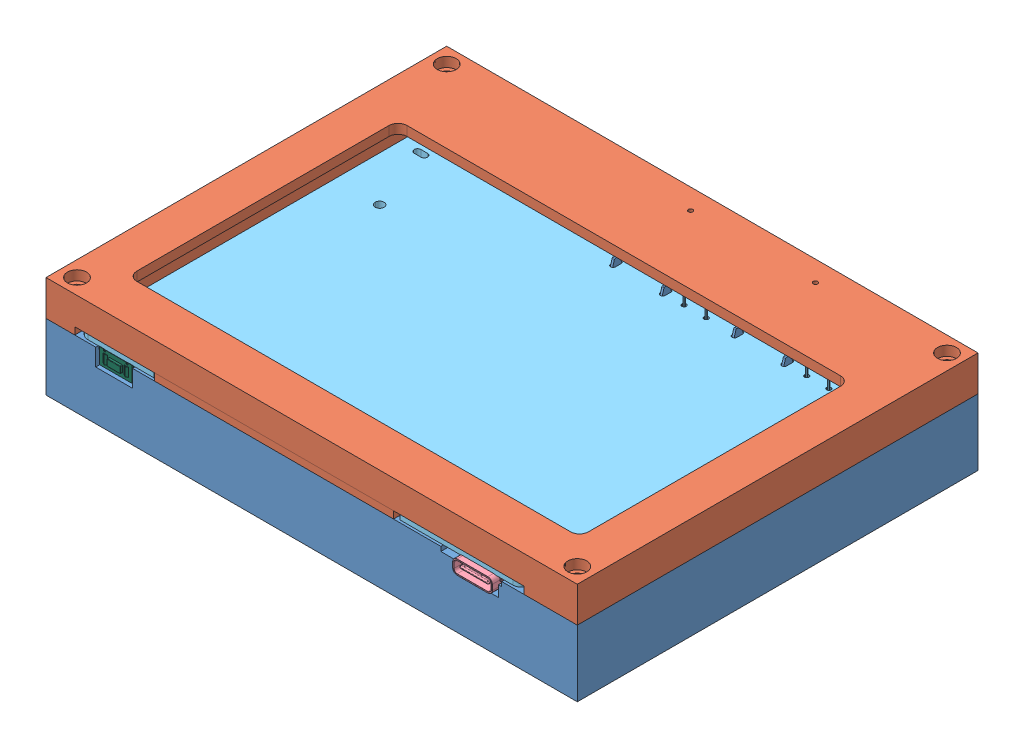
SolidWorks assembly 装配体2, configuration 默认. Lengths in mm. (continued)
Components (placement in the parent): (continued)
- 3D_board_2024-11-06-1: 3D_board_2024-11-06 [默认] at (-63.7814 -6.4105 44.7375) x (1 0 0) z (0 -1 0) size (99.97 100.01 16.2) (continued)
  - 3D_board_2024-11-06.step-1: 3D_board_2024-11-06.step [默认] at origin size (99.97 100.01 16.2) (continued)
    - iqks-C150.step-1: iqks-C150.step [默认] at (51.6811 -62.7701 1.5862) size (1.6 0.8 0.8)
      - C0603.step-1: C0603.step [默认] at origin size (1.6 0.8 0.8)
        - SOLID-10.step-1: SOLID-10.step [默认] at origin size (1.6 0.8 0.8)
    - iqks-C153.step-1: iqks-C153.step [默认] at (80.0102 -41.0211 1.5862) x (0 -1 0) z (0 0 1) size (1.6 0.8 0.8)
      - C0603.step-1: C0603.step [默认] at origin size (1.6 0.8 0.8)
        - SOLID-10.step-1: SOLID-10.step [默认] at origin size (1.6 0.8 0.8)
    - iqks-C15.step-1: iqks-C15.step [默认] at (71.7551 -65.8101 1.5862) x (0 1 0) z (0 0 1) size (1.6 0.8 0.8)
      - C0603.step-1: C0603.step [默认] at origin size (1.6 0.8 0.8)
        - SOLID-10.step-1: SOLID-10.step [默认] at origin size (1.6 0.8 0.8)
    - iqks-C16.step-1: iqks-C16.step [默认] at (83.1852 -65.8101 1.5862) x (0 1 0) z (0 0 1) size (1.6 0.8 0.8)
      - C0603.step-1: C0603.step [默认] at origin size (1.6 0.8 0.8)
        - SOLID-10.step-1: SOLID-10.step [默认] at origin size (1.6 0.8 0.8)
    - iqks-C38.step-1: iqks-C38.step [默认] at (85.7252 -65.8101 1.5862) x (0 1 0) z (0 0 1) size (1.6 0.8 0.8)
      - C0603.step-1: C0603.step [默认] at origin size (1.6 0.8 0.8)
        - SOLID-10.step-1: SOLID-10.step [默认] at origin size (1.6 0.8 0.8)
    - iqks-C39.step-1: iqks-C39.step [默认] at (97.1552 -65.8101 1.5862) x (0 1 0) z (0 0 1) size (1.6 0.8 0.8)
      - C0603.step-1: C0603.step [默认] at origin size (1.6 0.8 0.8)
        - SOLID-10.step-1: SOLID-10.step [默认] at origin size (1.6 0.8 0.8)
    - iqks-C17.step-1: iqks-C17.step [默认] at (26.6701 -67.3101 1.5862) x (0 -1 0) z (0 0 1) size (1.6 0.8 0.8)
      - C0603.step-1: C0603.step [默认] at origin size (1.6 0.8 0.8)
        - SOLID-10.step-1: SOLID-10.step [默认] at origin size (1.6 0.8 0.8)
    - iqks-C18.step-1: iqks-C18.step [默认] at (35.5601 -67.3101 1.5862) x (0 -1 0) z (0 0 1) size (1.6 0.8 0.8)
      - C0603.step-1: C0603.step [默认] at origin size (1.6 0.8 0.8)
        - SOLID-10.step-1: SOLID-10.step [默认] at origin size (1.6 0.8 0.8)
    - iqks-C50.step-1: iqks-C50.step [默认] at (12.065 -67.3101 1.5862) x (0 -1 0) z (0 0 1) size (1.6 0.8 0.8)
      - C0603.step-1: C0603.step [默认] at origin size (1.6 0.8 0.8)
        - SOLID-10.step-1: SOLID-10.step [默认] at origin size (1.6 0.8 0.8)
    - iqks-C51.step-1: iqks-C51.step [默认] at (20.955 -67.3101 1.5862) x (0 -1 0) z (0 0 1) size (1.6 0.8 0.8)
      - C0603.step-1: C0603.step [默认] at origin size (1.6 0.8 0.8)
        - SOLID-10.step-1: SOLID-10.step [默认] at origin size (1.6 0.8 0.8)
    - iqks-C22.step-1: iqks-C22.step [默认] at (17.78 -74.9301 1.5862) x (0 1 0) z (0 0 1) size (1.6 0.8 0.8)
      - C0603.step-1: C0603.step [默认] at origin size (1.6 0.8 0.8)
        - SOLID-10.step-1: SOLID-10.step [默认] at origin size (1.6 0.8 0.8)
    - iqks-C28.step-1: iqks-C28.step [默认] at (17.78 -71.1201 1.5862) x (0 -1 0) z (0 0 1) size (1.6 0.8 0.8)
      - C0603.step-1: C0603.step [默认] at origin size (1.6 0.8 0.8)
        - SOLID-10.step-1: SOLID-10.step [默认] at origin size (1.6 0.8 0.8)
    - iqks-C31.step-1: iqks-C31.step [默认] at (32.3851 -74.9301 1.5862) x (0 1 0) z (0 0 1) size (1.6 0.8 0.8)
      - C0603.step-1: C0603.step [默认] at origin size (1.6 0.8 0.8)
        - SOLID-10.step-1: SOLID-10.step [默认] at origin size (1.6 0.8 0.8)
    - iqks-C32.step-1: iqks-C32.step [默认] at (32.3851 -71.1201 1.5862) x (0 -1 0) z (0 0 1) size (1.6 0.8 0.8)
      - C0603.step-1: C0603.step [默认] at origin size (1.6 0.8 0.8)
        - SOLID-10.step-1: SOLID-10.step [默认] at origin size (1.6 0.8 0.8)
    - iqks-C113.step-1: iqks-C113.step [默认] at (53.8401 -57.5551 1.5862) x (0 1 0) z (0 0 1) size (1.6 0.8 0.8)
      - C0603.step-1: C0603.step [默认] at origin size (1.6 0.8 0.8)
        - SOLID-10.step-1: SOLID-10.step [默认] at origin size (1.6 0.8 0.8)
    - iqks-C116.step-1: iqks-C116.step [默认] at (38.1001 -59.0551 1.5862) x (0 1 0) z (0 0 1) size (1.6 0.8 0.8)
      - C0603.step-1: C0603.step [默认] at origin size (1.6 0.8 0.8)
        - SOLID-10.step-1: SOLID-10.step [默认] at origin size (1.6 0.8 0.8)
    - iqks-C25.step-1: iqks-C25.step [默认] at (63.1191 -60.9601 1.5862) x (-1 0 0) z (0 0 1) size (1.6 0.8 0.8)
      - C0603.step-1: C0603.step [默认] at origin size (1.6 0.8 0.8)
        - SOLID-10.step-1: SOLID-10.step [默认] at origin size (1.6 0.8 0.8)
    - iqks-C27.step-1: iqks-C27.step [默认] at (66.2941 -60.9601 1.5862) x (-1 0 0) z (0 0 1) size (1.6 0.8 0.8)
      - C0603.step-1: C0603.step [默认] at origin size (1.6 0.8 0.8)
        - SOLID-10.step-1: SOLID-10.step [默认] at origin size (1.6 0.8 0.8)
    - iqks-C129.step-1: iqks-C129.step [默认] at (58.0391 -59.6901 1.5862) x (0 1 0) z (0 0 1) size (1.6 0.8 0.8)
      - C0603.step-1: C0603.step [默认] at origin size (1.6 0.8 0.8)
        - SOLID-10.step-1: SOLID-10.step [默认] at origin size (1.6 0.8 0.8)
    - iqks-C154.step-1: iqks-C154.step [默认] at (60.3251 -50.8001 1.5862) x (0 -1 0) z (0 0 1) size (1.6 0.8 0.8)
      - C0603.step-1: C0603.step [默认] at origin size (1.6 0.8 0.8)
        - SOLID-10.step-1: SOLID-10.step [默认] at origin size (1.6 0.8 0.8)
    - iqks-C138.step-1: iqks-C138.step [默认] at (85.0902 -48.6411 1.5862) size (1.6 0.8 0.8)
      - C0603.step-1: C0603.step [默认] at origin size (1.6 0.8 0.8)
        - SOLID-10.step-1: SOLID-10.step [默认] at origin size (1.6 0.8 0.8)
    - iqks-C139.step-1: iqks-C139.step [默认] at (84.7092 -51.8161 1.5862) x (0 1 0) z (0 0 1) size (1.6 0.8 0.8)
      - C0603.step-1: C0603.step [默认] at origin size (1.6 0.8 0.8)
        - SOLID-10.step-1: SOLID-10.step [默认] at origin size (1.6 0.8 0.8)
    - iqks-C149.step-1: iqks-C149.step [默认] at (82.5502 -51.8161 1.5862) x (0 1 0) z (0 0 1) size (1.6 0.8 0.8)
      - C0603.step-1: C0603.step [默认] at origin size (1.6 0.8 0.8)
        - SOLID-10.step-1: SOLID-10.step [默认] at origin size (1.6 0.8 0.8)
    - iqks-C3.step-1: iqks-C3.step [默认] at (16.51 -64.1351 1.5862) x (-1 0 0) z (0 0 1) size (1.6 0.8 0.8)
      - C0603.step-1: C0603.step [默认] at origin size (1.6 0.8 0.8)
        - SOLID-10.step-1: SOLID-10.step [默认] at origin size (1.6 0.8 0.8)
    - iqks-C4.step-1: iqks-C4.step [默认] at (19.62 -64.1351 1.5862) size (1.6 0.8 0.8)
      - C0603.step-1: C0603.step [默认] at origin size (1.6 0.8 0.8)
        - SOLID-10.step-1: SOLID-10.step [默认] at origin size (1.6 0.8 0.8)
    - iqks-C5.step-1: iqks-C5.step [默认] at (13.335 -64.1351 1.5862) size (1.6 0.8 0.8)
      - C0603.step-1: C0603.step [默认] at origin size (1.6 0.8 0.8)
        - SOLID-10.step-1: SOLID-10.step [默认] at origin size (1.6 0.8 0.8)
    - iqks-C19.step-1: iqks-C19.step [默认] at (31.1151 -64.1351 1.5862) x (-1 0 0) z (0 0 1) size (1.6 0.8 0.8)
      - C0603.step-1: C0603.step [默认] at origin size (1.6 0.8 0.8)
        - SOLID-10.step-1: SOLID-10.step [默认] at origin size (1.6 0.8 0.8)
    - iqks-C20.step-1: iqks-C20.step [默认] at (34.225 -64.1351 1.5862) size (1.6 0.8 0.8)
      - C0603.step-1: C0603.step [默认] at origin size (1.6 0.8 0.8)
        - SOLID-10.step-1: SOLID-10.step [默认] at origin size (1.6 0.8 0.8)
    - iqks-C21.step-1: iqks-C21.step [默认] at (27.9401 -64.1351 1.5862) size (1.6 0.8 0.8)
      - C0603.step-1: C0603.step [默认] at origin size (1.6 0.8 0.8)
        - SOLID-10.step-1: SOLID-10.step [默认] at origin size (1.6 0.8 0.8)
    - iqks-C29.step-1: iqks-C29.step [默认] at (12.065 -70.4851 1.5862) size (1.6 0.8 0.8)
      - C0603.step-1: C0603.step [默认] at origin size (1.6 0.8 0.8)
        - SOLID-10.step-1: SOLID-10.step [默认] at origin size (1.6 0.8 0.8)
    - iqks-C30.step-1: iqks-C30.step [默认] at (15.24 -70.4851 1.5862) x (-1 0 0) z (0 0 1) size (1.6 0.8 0.8)
      - C0603.step-1: C0603.step [默认] at origin size (1.6 0.8 0.8)
        - SOLID-10.step-1: SOLID-10.step [默认] at origin size (1.6 0.8 0.8)
    - iqks-C33.step-1: iqks-C33.step [默认] at (26.6701 -70.4851 1.5862) size (1.6 0.8 0.8)
      - C0603.step-1: C0603.step [默认] at origin size (1.6 0.8 0.8)
        - SOLID-10.step-1: SOLID-10.step [默认] at origin size (1.6 0.8 0.8)
    - iqks-C36.step-1: iqks-C36.step [默认] at (29.8451 -70.4851 1.5862) x (-1 0 0) z (0 0 1) size (1.6 0.8 0.8)
      - C0603.step-1: C0603.step [默认] at origin size (1.6 0.8 0.8)
        - SOLID-10.step-1: SOLID-10.step [默认] at origin size (1.6 0.8 0.8)
    - iqks-C42.step-1: iqks-C42.step [默认] at (76.2002 -29.2101 1.5862) x (0 1 0) z (0 0 1) size (1.6 0.8 0.8)
      - C0603.step-1: C0603.step [默认] at origin size (1.6 0.8 0.8)
        - SOLID-10.step-1: SOLID-10.step [默认] at origin size (1.6 0.8 0.8)
    - iqks-C43.step-1: iqks-C43.step [默认] at (92.0752 -13.97 1.5862) x (0 1 0) z (0 0 1) size (1.6 0.8 0.8)
      - C0603.step-1: C0603.step [默认] at origin size (1.6 0.8 0.8)
        - SOLID-10.step-1: SOLID-10.step [默认] at origin size (1.6 0.8 0.8)
    - iqks-C44.step-1: iqks-C44.step [默认] at (93.8532 -15.113 1.5862) x (0 -1 0) z (0 0 1) size (1.6 0.8 0.8)
      - C0603.step-1: C0603.step [默认] at origin size (1.6 0.8 0.8)
        - SOLID-10.step-1: SOLID-10.step [默认] at origin size (1.6 0.8 0.8)
    - iqks-C46.step-1: iqks-C46.step [默认] at (78.1052 -29.2101 1.5862) x (0 1 0) z (0 0 1) size (1.6 0.8 0.8)
      - C0603.step-1: C0603.step [默认] at origin size (1.6 0.8 0.8)
        - SOLID-10.step-1: SOLID-10.step [默认] at origin size (1.6 0.8 0.8)
    - iqks-C49.step-1: iqks-C49.step [默认] at (93.9802 -27.9401 1.5862) x (-1 0 0) z (0 0 1) size (1.6 0.8 0.8)
      - C0603.step-1: C0603.step [默认] at origin size (1.6 0.8 0.8)
        - SOLID-10.step-1: SOLID-10.step [默认] at origin size (1.6 0.8 0.8)
    - iqks-C54.step-1: iqks-C54.step [默认] at (81.4072 -37.8461 1.5862) x (0 1 0) z (0 0 1) size (1.6 0.8 0.8)
      - C0603.step-1: C0603.step [默认] at origin size (1.6 0.8 0.8)
        - SOLID-10.step-1: SOLID-10.step [默认] at origin size (1.6 0.8 0.8)
    - iqks-C56.step-1: iqks-C56.step [默认] at (76.8352 -37.2111 1.5862) x (-1 0 0) z (0 0 1) size (1.6 0.8 0.8)
      - C0603.step-1: C0603.step [默认] at origin size (1.6 0.8 0.8)
        - SOLID-10.step-1: SOLID-10.step [默认] at origin size (1.6 0.8 0.8)
    - iqks-C61.step-1: iqks-C61.step [默认] at (56.1101 -65.3101 1.5862) x (0 1 0) z (0 0 1) size (1.6 0.8 0.8)
      - C0603.step-1: C0603.step [默认] at origin size (1.6 0.8 0.8)
        - SOLID-10.step-1: SOLID-10.step [默认] at origin size (1.6 0.8 0.8)
    - iqks-C134.step-1: iqks-C134.step [默认] at (75.5652 -24.765 1.5862) x (0 -1 0) z (0 0 1) size (1.6 0.8 0.8)
      - C0603.step-1: C0603.step [默认] at origin size (1.6 0.8 0.8)
        - SOLID-10.step-1: SOLID-10.step [默认] at origin size (1.6 0.8 0.8)
    - iqks-C135.step-1: iqks-C135.step [默认] at (84.4552 -27.3051 1.5862) x (0 -1 0) z (0 0 1) size (1.6 0.8 0.8)
      - C0603.step-1: C0603.step [默认] at origin size (1.6 0.8 0.8)
        - SOLID-10.step-1: SOLID-10.step [默认] at origin size (1.6 0.8 0.8)
    - iqks-C140.step-1: iqks-C140.step [默认] at (72.3901 -42.9261 1.5862) x (-1 0 0) z (0 0 1) size (1.6 0.8 0.8)
      - C0603.step-1: C0603.step [默认] at origin size (1.6 0.8 0.8)
        - SOLID-10.step-1: SOLID-10.step [默认] at origin size (1.6 0.8 0.8)
    - iqks-C141.step-1: iqks-C141.step [默认] at (72.3901 -41.0211 1.5862) x (-1 0 0) z (0 0 1) size (1.6 0.8 0.8)
      - C0603.step-1: C0603.step [默认] at origin size (1.6 0.8 0.8)
        - SOLID-10.step-1: SOLID-10.step [默认] at origin size (1.6 0.8 0.8)
    - iqks-C146.step-1: iqks-C146.step [默认] at (90.0432 -46.1011 1.5862) x (0 -1 0) z (0 0 1) size (1.6 0.8 0.8)
      - C0603.step-1: C0603.step [默认] at origin size (1.6 0.8 0.8)
        - SOLID-10.step-1: SOLID-10.step [默认] at origin size (1.6 0.8 0.8)
    - iqks-C147.step-1: iqks-C147.step [默认] at (91.9482 -46.1011 1.5862) x (0 1 0) z (0 0 1) size (1.6 0.8 0.8)
      - C0603.step-1: C0603.step [默认] at origin size (1.6 0.8 0.8)
        - SOLID-10.step-1: SOLID-10.step [默认] at origin size (1.6 0.8 0.8)
    - iqks-C151.step-1: iqks-C151.step [默认] at (49.7601 -65.3101 1.5862) x (0 -1 0) z (0 0 1) size (1.6 0.8 0.8)
      - C0603.step-1: C0603.step [默认] at origin size (1.6 0.8 0.8)
        - SOLID-10.step-1: SOLID-10.step [默认] at origin size (1.6 0.8 0.8)
    - iqks-C156.step-1: iqks-C156.step [默认] at (64.4229 -42.0779 1.5862) x (0 -1 0) z (0 0 1) size (1.6 0.8 0.8)
      - C0603.step-1: C0603.step [默认] at origin size (1.6 0.8 0.8)
        - SOLID-10.step-1: SOLID-10.step [默认] at origin size (1.6 0.8 0.8)
    - iqks-C159.step-1: iqks-C159.step [默认] at (93.8532 -46.4821 1.5862) x (0 -1 0) z (0 0 1) size (1.6 0.8 0.8)
      - C0603.step-1: C0603.step [默认] at origin size (1.6 0.8 0.8)
        - SOLID-10.step-1: SOLID-10.step [默认] at origin size (1.6 0.8 0.8)
    - iqks-C162.step-1: iqks-C162.step [默认] at (93.8532 -42.7991 1.5862) x (0 -1 0) z (0 0 1) size (1.6 0.8 0.8)
      - C0603.step-1: C0603.step [默认] at origin size (1.6 0.8 0.8)
        - SOLID-10.step-1: SOLID-10.step [默认] at origin size (1.6 0.8 0.8)
    - iqks-C163.step-1: iqks-C163.step [默认] at (64.4229 -38.7759 1.5862) x (0 -1 0) z (0 0 1) size (1.6 0.8 0.8)
      - C0603.step-1: C0603.step [默认] at origin size (1.6 0.8 0.8)
        - SOLID-10.step-1: SOLID-10.step [默认] at origin size (1.6 0.8 0.8)
    - iqks-C1.step-1: iqks-C1.step [默认] at (54.2011 -18.923 1.5862) size (1.6 0.8 0.8)
      - C0603.step-1: C0603.step [默认] at origin size (1.6 0.8 0.8)
        - SOLID-10.step-1: SOLID-10.step [默认] at origin size (1.6 0.8 0.8)
    - iqks-C2.step-1: iqks-C2.step [默认] at (51.5621 -18.0991 1.5862) x (0 1 0) z (0 0 1) size (1.6 0.8 0.8)
      - C0603.step-1: C0603.step [默认] at origin size (1.6 0.8 0.8)
        - SOLID-10.step-1: SOLID-10.step [默认] at origin size (1.6 0.8 0.8)
    - iqks-C57.step-1: iqks-C57.step [默认] at (86.3602 -46.1011 1.5862) x (0 -1 0) z (0 0 1) size (1.6 0.8 0.8)
      - C0603.step-1: C0603.step [默认] at origin size (1.6 0.8 0.8)
        - SOLID-10.step-1: SOLID-10.step [默认] at origin size (1.6 0.8 0.8)
    - iqks-C94.step-1: iqks-C94.step [默认] at (53.9751 -49.1491 1.5862) size (1.6 0.8 0.8)
      - C0603.step-1: C0603.step [默认] at origin size (1.6 0.8 0.8)
        - SOLID-10.step-1: SOLID-10.step [默认] at origin size (1.6 0.8 0.8)
    - iqks-C95.step-1: iqks-C95.step [默认] at (50.8001 -46.3551 1.5862) x (0 -1 0) z (0 0 1) size (1.6 0.8 0.8)
      - C0603.step-1: C0603.step [默认] at origin size (1.6 0.8 0.8)
        - SOLID-10.step-1: SOLID-10.step [默认] at origin size (1.6 0.8 0.8)
    - iqks-C96.step-1: iqks-C96.step [默认] at (60.9601 -64.1351 1.5862) x (0 1 0) z (0 0 1) size (1.6 0.8 0.8)
      - C0603.step-1: C0603.step [默认] at origin size (1.6 0.8 0.8)
        - SOLID-10.step-1: SOLID-10.step [默认] at origin size (1.6 0.8 0.8)
    - iqks-C97.step-1: iqks-C97.step [默认] at (67.3101 -64.1351 1.5862) x (0 1 0) z (0 0 1) size (1.6 0.8 0.8)
      - C0603.step-1: C0603.step [默认] at origin size (1.6 0.8 0.8)
        - SOLID-10.step-1: SOLID-10.step [默认] at origin size (1.6 0.8 0.8)
    - iqks-C148.step-1: iqks-C148.step [默认] at (76.8352 -51.8161 1.5862) x (0 -1 0) z (0 0 1) size (1.6 0.8 0.8)
      - C0603.step-1: C0603.step [默认] at origin size (1.6 0.8 0.8)
        - SOLID-10.step-1: SOLID-10.step [默认] at origin size (1.6 0.8 0.8)
    - iqks-C164.step-1: iqks-C164.step [默认] at (66.4211 -44.4501 1.5862) x (-1 0 0) z (0 0 1) size (1.6 0.8 0.8)
      - C0603.step-1: C0603.step [默认] at origin size (1.6 0.8 0.8)
        - SOLID-10.step-1: SOLID-10.step [默认] at origin size (1.6 0.8 0.8)
    - iqks-C165.step-1: iqks-C165.step [默认] at (94.8692 -49.0221 1.5862) x (-1 0 0) z (0 0 1) size (1.6 0.8 0.8)
      - C0603.step-1: C0603.step [默认] at origin size (1.6 0.8 0.8)
        - SOLID-10.step-1: SOLID-10.step [默认] at origin size (1.6 0.8 0.8)
    - iqks-C166.step-1: iqks-C166.step [默认] at (70.4851 -38.2271 1.5862) x (-1 0 0) z (0 0 1) size (1.6 0.8 0.8)
      - C0603.step-1: C0603.step [默认] at origin size (1.6 0.8 0.8)
        - SOLID-10.step-1: SOLID-10.step [默认] at origin size (1.6 0.8 0.8)
    - iqks-C167.step-1: iqks-C167.step [默认] at (96.1392 -39.8781 1.5862) size (1.6 0.8 0.8)
      - C0603.step-1: C0603.step [默认] at origin size (1.6 0.8 0.8)
        - SOLID-10.step-1: SOLID-10.step [默认] at origin size (1.6 0.8 0.8)
    - iqks-C168.step-1: iqks-C168.step [默认] at (49.4103 -33.4035 1.5862) size (1.6 0.8 0.8)
      - C0603.step-1: C0603.step [默认] at origin size (1.6 0.8 0.8)
        - SOLID-10.step-1: SOLID-10.step [默认] at origin size (1.6 0.8 0.8)
    - iqks-C169.step-1: iqks-C169.step [默认] at (90.9728 -30.8843 1.5862) x (0 1 0) z (0 0 1) size (1.6 0.8 0.8)
      - C0603.step-1: C0603.step [默认] at origin size (1.6 0.8 0.8)
        - SOLID-10.step-1: SOLID-10.step [默认] at origin size (1.6 0.8 0.8)
    - iqks-C173.step-1: iqks-C173.step [默认] at (78.3514 -14.0943 1.5862) x (-1 0 0) z (0 0 1) size (1.6 0.8 0.8)
      - C0603.step-1: C0603.step [默认] at origin size (1.6 0.8 0.8)
        - SOLID-10.step-1: SOLID-10.step [默认] at origin size (1.6 0.8 0.8)
    - iqks-C174.step-1: iqks-C174.step [默认] at (5.969 -10.414 1.5862) size (1.6 0.8 0.8)
      - C0603.step-1: C0603.step [默认] at origin size (1.6 0.8 0.8)
        - SOLID-10.step-1: SOLID-10.step [默认] at origin size (1.6 0.8 0.8)
    - iqks-C9.step-1: iqks-C9.step [默认] at (71.3741 -84.1142 1.5862) x (-1 0 0) z (0 0 1) size (1.6 0.8 0.8)
      - C0603.step-1: C0603.step [默认] at origin size (1.6 0.8 0.8)
        - SOLID-10.step-1: SOLID-10.step [默认] at origin size (1.6 0.8 0.8)
    - iqks-C52.step-1: iqks-C52.step [默认] at (64.0081 -84.1142 1.5862) size (1.6 0.8 0.8)
      - C0603.step-1: C0603.step [默认] at origin size (1.6 0.8 0.8)
        - SOLID-10.step-1: SOLID-10.step [默认] at origin size (1.6 0.8 0.8)
    - iqks-C115.step-1: iqks-C115.step [默认] at (48.8951 -61.5951 1.5862) x (0 -1 0) z (0 0 1) size (1.6 0.8 0.8)
      - C0603.step-1: C0603.step [默认] at origin size (1.6 0.8 0.8)
        - SOLID-10.step-1: SOLID-10.step [默认] at origin size (1.6 0.8 0.8)
    - iqks-D2.step-1: iqks-D2.step [默认] at (86.9952 -42.9261 1.5862) x (-1 0 0) z (0 0 1) size (5.21 2.62 2.16)
      - SMA_L4.2-W2.6-LS5.3-RD.step-1: SMA_L4.2-W2.6-LS5.3-RD.step [默认] at origin size (5.21 2.62 2.16)
        - COMPOUND-11.step-1: COMPOUND-11.step [默认] at origin size (5.21 2.62 2.16)
    - iqks-D3.step-1: iqks-D3.step [默认] at (76.2002 -46.3551 1.5862) x (0 1 0) z (0 0 1) size (5.21 2.62 2.16)
      - SMA_L4.2-W2.6-LS5.3-RD.step-1: SMA_L4.2-W2.6-LS5.3-RD.step [默认] at origin size (5.21 2.62 2.16)
        - COMPOUND-11.step-1: COMPOUND-11.step [默认] at origin size (5.21 2.62 2.16)
    - iqks-D1.step-1: iqks-D1.step [默认] at (89.2812 -20.955 1.5862) x (0 1 0) z (0 0 1) size (5.21 2.62 2.16)
      - SMA_L4.2-W2.6-LS5.3-RD.step-1: SMA_L4.2-W2.6-LS5.3-RD.step [默认] at origin size (5.21 2.62 2.16)
        - COMPOUND-11.step-1: COMPOUND-11.step [默认] at origin size (5.21 2.62 2.16)
    - iqks-U17.step-1: iqks-U17.step [默认] at (10.7362 -45.5718 1.5862) size (2.81 2.9 1.65)
      - SOT-23-6_L2.9-W1.6-P0.95-LS2.8-BR.step-1: SOT-23-6_L2.9-W1.6-P0.95-LS2.8-BR.step [默认] at origin size (2.81 2.9 1.65)
        - COMPOUND-12.step-1: COMPOUND-12.step [默认] at origin size (2.81 2.9 1.65)
    - iqks-J4.step-1: iqks-J4.step [默认] at (30.8651 -83.1852 1.5862) size (7.9 14.5 5.75)
      - AUDIO-SMD_PJ-393.step-1: AUDIO-SMD_PJ-393.step [默认] at origin size (7.9 14.5 5.75)
        - COMPOUND-13.step-1: COMPOUND-13.step [默认] at origin size (7.9 14.5 5.75)
    - iqks-J5.step-1: iqks-J5.step [默认] at (16.51 -83.1852 1.5862) size (7.9 14.5 5.75)
      - AUDIO-SMD_PJ-393.step-1: AUDIO-SMD_PJ-393.step [默认] at origin size (7.9 14.5 5.75)
        - COMPOUND-13.step-1: COMPOUND-13.step [默认] at origin size (7.9 14.5 5.75)
    - iqks-Q6.step-1: iqks-Q6.step [默认] at (84.2012 -20.955 1.5862) x (0 1 0) z (0 0 1) size (2.8 2.7 1.35)
      - SOT-23-3_L2.9-W1.6-P1.90-LS2.8-BR.step-1: SOT-23-3_L2.9-W1.6-P1.90-LS2.8-BR.step [默认] at origin size (2.8 2.7 1.35)
        - SOLID-14.step-1: SOLID-14.step [默认] at origin size (2.8 2.7 1.35)
    - iqks-Q7.step-1: iqks-Q7.step [默认] at (89.5352 -27.3051 1.5862) x (-1 0 0) z (0 0 1) size (2.8 2.7 1.35)
      - SOT-23-3_L2.9-W1.6-P1.90-LS2.8-BR.step-1: SOT-23-3_L2.9-W1.6-P1.90-LS2.8-BR.step [默认] at origin size (2.8 2.7 1.35)
        - SOLID-14.step-1: SOLID-14.step [默认] at origin size (2.8 2.7 1.35)
    - iqks-Q8.step-1: iqks-Q8.step [默认] at (80.6452 -27.3051 1.5862) size (2.8 2.7 1.35)
      - SOT-23-3_L2.9-W1.6-P1.90-LS2.8-BR.step-1: SOT-23-3_L2.9-W1.6-P1.90-LS2.8-BR.step [默认] at origin size (2.8 2.7 1.35)
        - SOLID-14.step-1: SOLID-14.step [默认] at origin size (2.8 2.7 1.35)
    - iqks-Q5.step-1: iqks-Q5.step [默认] at (77.4702 -34.4171 1.5862) x (-1 0 0) z (0 0 1) size (2.8 2.7 1.35)
      - SOT-23-3_L2.9-W1.6-P1.90-LS2.8-BR.step-1: SOT-23-3_L2.9-W1.6-P1.90-LS2.8-BR.step [默认] at origin size (2.8 2.7 1.35)
        - SOLID-14.step-1: SOLID-14.step [默认] at origin size (2.8 2.7 1.35)
    - iqks-U27.step-1: iqks-U27.step [默认] at (80.6452 -46.1011 1.5862) x (0 -1 0) z (0 0 1) size (4.02 4.02 0.92)
      - QFN-24_L4.0-W4.0-P0.50-TL-EP2.6.step-1: QFN-24_L4.0-W4.0-P0.50-TL-EP2.6.step [默认] at origin size (4.02 4.02 0.92)
        - SOLID-15.step-1: SOLID-15.step [默认] at origin size (4.02 4.02 0.92)
    - iqks-L4.step-1: iqks-L4.step [默认] at (89.5352 -14.605 1.5862) x (0 1 0) z (0 0 1) size (2 1.3 0.61)
      - L0805.step-1: L0805.step [默认] at origin size (2 1.3 0.61)
        - COMPOUND-16.step-1: COMPOUND-16.step [默认] at origin size (2 1.3 0.61)
    - iqks-J3.step-1: iqks-J3.step [默认] at (90.1702 -3.81 1.5862) x (-1 0 0) z (0 0 1) size (8.94 7.9 4.1)
      - usb-c_smd-type-c-31-m-12.step-1: usb-c_smd-type-c-31-m-12.step [默认] at origin size (8.94 7.9 4.1)
        - COMPOUND-17.step-1: COMPOUND-17.step [默认] at origin size (8.94 7.9 4.1)
    - iqks-U15.step-1: iqks-U15.step [默认] at (46.9901 -38.7351 1.5862) size (5 6.41 1.05)
      - TSSOP-16_L5.0-W4.4-P0.65-LS6.4-BL.step-1: TSSOP-16_L5.0-W4.4-P0.65-LS6.4-BL.step [默认] at origin size (5 6.41 1.05)
        - COMPOUND-18.step-1: COMPOUND-18.step [默认] at origin size (5 6.41 1.05)
    - iqks-LED3.step-1: iqks-LED3.step [默认] at (52.7051 -80.7722 0) x (1 0 0) z (0 0 -1) size (2.01 1.25 1)
      - LED_0805.step-1: LED_0805.step [默认] at origin size (2.01 1.25 1)
        - COMPOUND-19.step-1: COMPOUND-19.step [默认] at origin size (2.01 1.25 1)
    - iqks-LED2.step-1: iqks-LED2.step [默认] at (80.8992 -80.7722 0) x (1 0 0) z (0 0 -1) size (2.01 1.25 1)
      - LED_0805.step-1: LED_0805.step [默认] at origin size (2.01 1.25 1)
        - COMPOUND-19.step-1: COMPOUND-19.step [默认] at origin size (2.01 1.25 1)
    - iqks-L9.step-1: iqks-L9.step [默认] at (49.4103 -31.4985 1.5862) size (1.62 0.82 0.82)
      - BEAD-SMD_L1.6-W0.8-P1.6.step-1: BEAD-SMD_L1.6-W0.8-P1.6.step [默认] at origin size (1.62 0.82 0.82)
        - SOLID-20.step-1: SOLID-20.step [默认] at origin size (1.62 0.82 0.82)
    - iqks-L10.step-1: iqks-L10.step [默认] at (53.0081 -60.0001 1.5862) size (1.62 0.82 0.82)
      - BEAD-SMD_L1.6-W0.8-P1.6.step-1: BEAD-SMD_L1.6-W0.8-P1.6.step [默认] at origin size (1.62 0.82 0.82)
        - SOLID-20.step-1: SOLID-20.step [默认] at origin size (1.62 0.82 0.82)
    - iqks-L11.step-1: iqks-L11.step [默认] at (39.3701 -62.2301 1.5862) x (-1 0 0) z (0 0 1) size (1.62 0.82 0.82)
      - BEAD-SMD_L1.6-W0.8-P1.6.step-1: BEAD-SMD_L1.6-W0.8-P1.6.step [默认] at origin size (1.62 0.82 0.82)
        - SOLID-20.step-1: SOLID-20.step [默认] at origin size (1.62 0.82 0.82)
    - iqks-L6.step-1: iqks-L6.step [默认] at (12.7 -14.478 1.5862) x (0 -1 0) z (0 0 1) size (1.62 0.82 0.82)
      - BEAD-SMD_L1.6-W0.8-P1.6.step-1: BEAD-SMD_L1.6-W0.8-P1.6.step [默认] at origin size (1.62 0.82 0.82)
        - SOLID-20.step-1: SOLID-20.step [默认] at origin size (1.62 0.82 0.82)
    - iqks-LDO1.step-1: iqks-LDO1.step [默认] at (54.2011 -16.383 1.5862) x (0 1 0) z (0 0 1) size (2.9 3.01 1.25)
      - SOT-23-5_L3.0-W1.7-P0.95-LS2.8-BL.step-1: SOT-23-5_L3.0-W1.7-P0.95-LS2.8-BL.step [默认] at origin size (2.9 3.01 1.25)
        - COMPOUND-21.step-1: COMPOUND-21.step [默认] at origin size (2.9 3.01 1.25)
    - iqks-LDO2.step-1: iqks-LDO2.step [默认] at (53.9751 -46.3551 1.5862) x (0 1 0) z (0 0 1) size (2.9 3.01 1.25)
      - SOT-23-5_L3.0-W1.7-P0.95-LS2.8-BL.step-1: SOT-23-5_L3.0-W1.7-P0.95-LS2.8-BL.step [默认] at origin size (2.9 3.01 1.25)
        - COMPOUND-21.step-1: COMPOUND-21.step [默认] at origin size (2.9 3.01 1.25)
    - iqks-LDO3.step-1: iqks-LDO3.step [默认] at (64.3026 -64.2217 1.5862) x (0 -1 0) z (0 0 1) size (2.9 3.01 1.25)
      - SOT-23-5_L3.0-W1.7-P0.95-LS2.8-BL.step-1: SOT-23-5_L3.0-W1.7-P0.95-LS2.8-BL.step [默认] at origin size (2.9 3.01 1.25)
        - COMPOUND-21.step-1: COMPOUND-21.step [默认] at origin size (2.9 3.01 1.25)
    - iqks-U28.step-1: iqks-U28.step [默认] at (52.9351 -65.4371 1.5862) x (0 1 0) z (0 0 1) size (2.9 3.01 1.25)
      - SOT-23-5_L3.0-W1.7-P0.95-LS2.8-BL.step-1: SOT-23-5_L3.0-W1.7-P0.95-LS2.8-BL.step [默认] at origin size (2.9 3.01 1.25)
        - COMPOUND-21.step-1: COMPOUND-21.step [默认] at origin size (2.9 3.01 1.25)
    - iqks-D10.step-1: iqks-D10.step [默认] at (9.779 -4.445 1.5862) size (2.51 1.3 1.2)
      - SOD-323_L1.8-W1.3-LS2.5-RD.step-1: SOD-323_L1.8-W1.3-LS2.5-RD.step [默认] at origin size (2.51 1.3 1.2)
        - COMPOUND-22.step-1: COMPOUND-22.step [默认] at origin size (2.51 1.3 1.2)
    - iqks-D9.step-1: iqks-D9.step [默认] at (9.779 -6.35 1.5862) size (2.51 1.3 1.2)
      - SOD-323_L1.8-W1.3-LS2.5-RD.step-1: SOD-323_L1.8-W1.3-LS2.5-RD.step [默认] at origin size (2.51 1.3 1.2)
        - COMPOUND-22.step-1: COMPOUND-22.step [默认] at origin size (2.51 1.3 1.2)
    - iqks-U5.step-1: iqks-U5.step [默认] at (64.3891 -55.2451 1.5862) x (-1 0 0) z (0 0 1) size (3 3 0.72)
      - WQFN-20_L3.0-W3.0-P0.50-TL-EP1.4.step-1: WQFN-20_L3.0-W3.0-P0.50-TL-EP1.4.step [默认] at origin size (3 3 0.72)
        - COMPOUND-23.step-1: COMPOUND-23.step [默认] at origin size (3 3 0.72)
    - iqks-U26.step-1: iqks-U26.step [默认] at (93.9802 -20.955 1.5862) x (-1 0 0) z (0 0 1) size (4.81 6 1.72)
      - SOIC-8_L4.9-W3.9-P1.27-LS6.0-BL-EP.step-1: SOIC-8_L4.9-W3.9-P1.27-LS6.0-BL-EP.step [默认] at origin size (4.81 6 1.72)
        - COMPOUND-24.step-1: COMPOUND-24.step [默认] at origin size (4.81 6 1.72)
    - iqks-B1.step-1: iqks-B1.step [默认] at (70.4851 -19.685 1.5862) x (0 -1 0) z (0 0 1) size (7.9 8.6 5.5)
      - CONN-SMD_P2.00_S2B-PH-SM4-TB-LF-SN.step-1: CONN-SMD_P2.00_S2B-PH-SM4-TB-LF-SN.step [默认] at origin size (7.9 8.6 5.5)
        - COMPOUND-25.step-1: COMPOUND-25.step [默认] at origin size (7.9 8.6 5.5)
    - iqks-U25.step-1: iqks-U25.step [默认] at (79.3752 -19.05 1.5862) x (-1 0 0) z (0 0 1) size (4.9 6.1 1.7)
      - ESOP-8_L4.9-W3.9-P1.27-LS6.0-BL-EP.step-1: ESOP-8_L4.9-W3.9-P1.27-LS6.0-BL-EP.step [默认] at origin size (4.9 6.1 1.7)
        - COMPOUND-26.step-1: COMPOUND-26.step [默认] at origin size (4.9 6.1 1.7)
    - iqks-U7.step-1: iqks-U7.step [默认] at (71.1201 -27.3051 1.5862) x (0 -1 0) z (0 0 1) size (4.9 6.1 1.7)
      - ESOP-8_L4.9-W3.9-P1.27-LS6.0-BL-EP.step-1: ESOP-8_L4.9-W3.9-P1.27-LS6.0-BL-EP.step [默认] at origin size (4.9 6.1 1.7)
        - COMPOUND-26.step-1: COMPOUND-26.step [默认] at origin size (4.9 6.1 1.7)
    - iqks-U14.step-1: iqks-U14.step [默认] at (43.6881 -13.843 1.5862) x (-0.707107 0.707107 0) z (0 0 1) size (12.5 9 1)
      - LGA-16_L12.5-W9.0-P1.27-TL-EP.step-1: LGA-16_L12.5-W9.0-P1.27-TL-EP.step [默认] at origin size (12.5 9 1)
        - SOLID-27.step-1: SOLID-27.step [默认] at origin size (12.5 9 1)
    - iqks-SW1.step-1: iqks-SW1.step [默认] at (8.382 -1.778 1.5862) x (-1 0 0) z (0 0 1) size (7.7 3.7 4.3)
      - SW-SMD_SHOU_TS36CA-0.6.step-1: SW-SMD_SHOU_TS36CA-0.6.step [默认] at origin size (7.7 3.7 4.3)
        - COMPOUND-28.step-1: COMPOUND-28.step [默认] at origin size (7.7 3.7 4.3)
    - iqks-C111.step-1: iqks-C111.step [默认] at (46.9901 -62.8651 1.5862) x (0 1 0) z (0 0 1) size (3.2 1.6 1.3)
      - C1206.step-1: C1206.step [默认] at origin size (3.2 1.6 1.3)
        - SOLID-29.step-1: SOLID-29.step [默认] at origin size (3.2 1.6 1.3)
    - iqks-C112.step-1: iqks-C112.step [默认] at (44.4501 -62.8651 1.5862) x (0 1 0) z (0 0 1) size (3.2 1.6 1.3)
      - C1206.step-1: C1206.step [默认] at origin size (3.2 1.6 1.3)
        - SOLID-29.step-1: SOLID-29.step [默认] at origin size (3.2 1.6 1.3)
    - iqks-U3.step-1: iqks-U3.step [默认] at (30.9881 -67.3101 1.5862) x (0 -1 0) z (0 0 1) size (3 1.84 0.67)
      - MSOP-8_L3.0-W3.0-P0.65-LS5.0-BL-EP.step-1: MSOP-8_L3.0-W3.0-P0.65-LS5.0-BL-EP.step [默认] at origin size (3 1.84 0.67)
        - COMPOUND-30.step-1: COMPOUND-30.step [默认] at origin size (3 1.84 0.67)
    - iqks-U6.step-1: iqks-U6.step [默认] at (77.5031 -61.9746 1.5862) x (0 1 0) z (0 0 1) size (3 1.84 0.67)
      - MSOP-8_L3.0-W3.0-P0.65-LS5.0-BL-EP.step-1: MSOP-8_L3.0-W3.0-P0.65-LS5.0-BL-EP.step [默认] at origin size (3 1.84 0.67)
        - COMPOUND-30.step-1: COMPOUND-30.step [默认] at origin size (3 1.84 0.67)
    - iqks-U24.step-1: iqks-U24.step [默认] at (16.4771 -67.3117 1.5862) x (0 -1 0) z (0 0 1) size (3 1.84 0.67)
      - MSOP-8_L3.0-W3.0-P0.65-LS5.0-BL-EP.step-1: MSOP-8_L3.0-W3.0-P0.65-LS5.0-BL-EP.step [默认] at origin size (3 1.84 0.67)
        - COMPOUND-30.step-1: COMPOUND-30.step [默认] at origin size (3 1.84 0.67)
    - iqks-U2.step-1: iqks-U2.step [默认] at (91.2191 -61.9746 1.5862) x (0 1 0) z (0 0 1) size (3 1.84 0.67)
      - MSOP-8_L3.0-W3.0-P0.65-LS5.0-BL-EP.step-1: MSOP-8_L3.0-W3.0-P0.65-LS5.0-BL-EP.step [默认] at origin size (3 1.84 0.67)
        - COMPOUND-30.step-1: COMPOUND-30.step [默认] at origin size (3 1.84 0.67)
    - iqks-LED1.step-1: iqks-LED1.step [默认] at (83.8252 -2.607 1.5862) x (0 1 0) z (0 0 1) size (2.02 1.26 1.01)
      - LED0805-RD_RED.step-1: LED0805-RD_RED.step [默认] at origin size (2.02 1.26 1.01)
        - COMPOUND-31.step-1: COMPOUND-31.step [默认] at origin size (2.02 1.26 1.01)
    - iqks-J2.step-1: iqks-J2.step [默认] at (54.0001 -79.3092 1.5862) x (0 -1 0) z (0 0 1) size (33.1 15.8 15.7)
      - AUDIO-TH_PJ-611E.step-1: AUDIO-TH_PJ-611E.step [默认] at origin size (33.1 15.8 15.7)
        - COMPOUND-32.step-1: COMPOUND-32.step [默认] at origin size (33.1 15.8 15.7)
    - iqks-J1.step-1: iqks-J1.step [默认] at (81.5002 -79.2542 1.5862) x (0 -1 0) z (0 0 1) size (33.1 15.8 15.7)
      - AUDIO-TH_PJ-611E.step-1: AUDIO-TH_PJ-611E.step [默认] at origin size (33.1 15.8 15.7)
        - COMPOUND-32.step-1: COMPOUND-32.step [默认] at origin size (33.1 15.8 15.7)
    - iqks-Q9.step-1: iqks-Q9.step [默认] at (5.588 -7.493 1.5862) size (2.5 2.89 1.05)
      - SOT-23-3_L2.9-W1.3-P1.90-LS2.4-BR.step-1: SOT-23-3_L2.9-W1.3-P1.90-LS2.4-BR.step [默认] at origin size (2.5 2.89 1.05)
        - COMPOUND-33.step-1: COMPOUND-33.step [默认] at origin size (2.5 2.89 1.05)
    - iqks-U4.step-1: iqks-U4.step [默认] at (27.9401 -73.0251 1.5862) x (0 1 0) z (0 0 1) size (3 5.01 1.25)
      - VSSOP-8_L3.0-W3.0-P0.65-LS5.0-BL.step-1: VSSOP-8_L3.0-W3.0-P0.65-LS5.0-BL.step [默认] at origin size (3 5.01 1.25)
        - COMPOUND-34.step-1: COMPOUND-34.step [默认] at origin size (3 5.01 1.25)
    - iqks-U1.step-1: iqks-U1.step [默认] at (13.335 -73.0251 1.5862) x (0 1 0) z (0 0 1) size (3 5.01 1.25)
      - VSSOP-8_L3.0-W3.0-P0.65-LS5.0-BL.step-1: VSSOP-8_L3.0-W3.0-P0.65-LS5.0-BL.step [默认] at origin size (3 5.01 1.25)
        - COMPOUND-34.step-1: COMPOUND-34.step [默认] at origin size (3 5.01 1.25)
    - iqks-U12.step-1: iqks-U12.step [默认] at (29.5923 -19.1353 1.5862) x (-0.707107 -0.707107 0) z (0 0 1) size (16 16 1.5)
      - LQFP-100_L14.0-W14.0-P0.50-LS16.0-BL.step-1: LQFP-100_L14.0-W14.0-P0.50-LS16.0-BL.step [默认] at origin size (16 16 1.5)
        - SOLID-35.step-1: SOLID-35.step [默认] at origin size (16 16 1.5)
    - Board.step-1: Board.step [默认] at origin size (99.97 89.97 1.59)
Mates (geometry in assembly coordinates):
- 同心1: concentric: cylinder of 底板-1 through (-67.1932 -8.0305 41.75) axis (0 1 0) radius 0.8; cylinder of 面板-1 through (-67.1932 -8.0305 41.75) axis (0 1 0) radius 1.25
- 同心2: concentric: cylinder of 底板-1 through (45.8068 -8.0305 41.75) axis (0 1 0) radius 0.8; cylinder of 面板-1 through (45.8068 -8.0305 41.75) axis (0 1 0) radius 1.25
- 距离1: distance = 0 mm: plane of 面板-1 through (-70.6931 -8.0305 -45.2499) normal (0 -1 0); plane of 底板-1 through (-70.6931 -8.0305 -45.2499) normal (0 1 0)
- 重合1: coincident: plane of 面板-1 through (-10.6932 -6.4105 0) normal (0 -1 0); plane of 3D_board_2024-11-06-1/3D_board_2024-11-06.step-1/Board.step-1 through (-13.9031 -6.4105 -0.0395) normal (0 1 0)
- 重合2: coincident: plane of 面板-1 through (49.3067 -8.0305 -45.25) normal (0 0 -1); plane of 3D_board_2024-11-06-1/3D_board_2024-11-06.step-1/Board.step-1 through (34.2188 -6.4105 -45.25) normal (0 0 -1)
